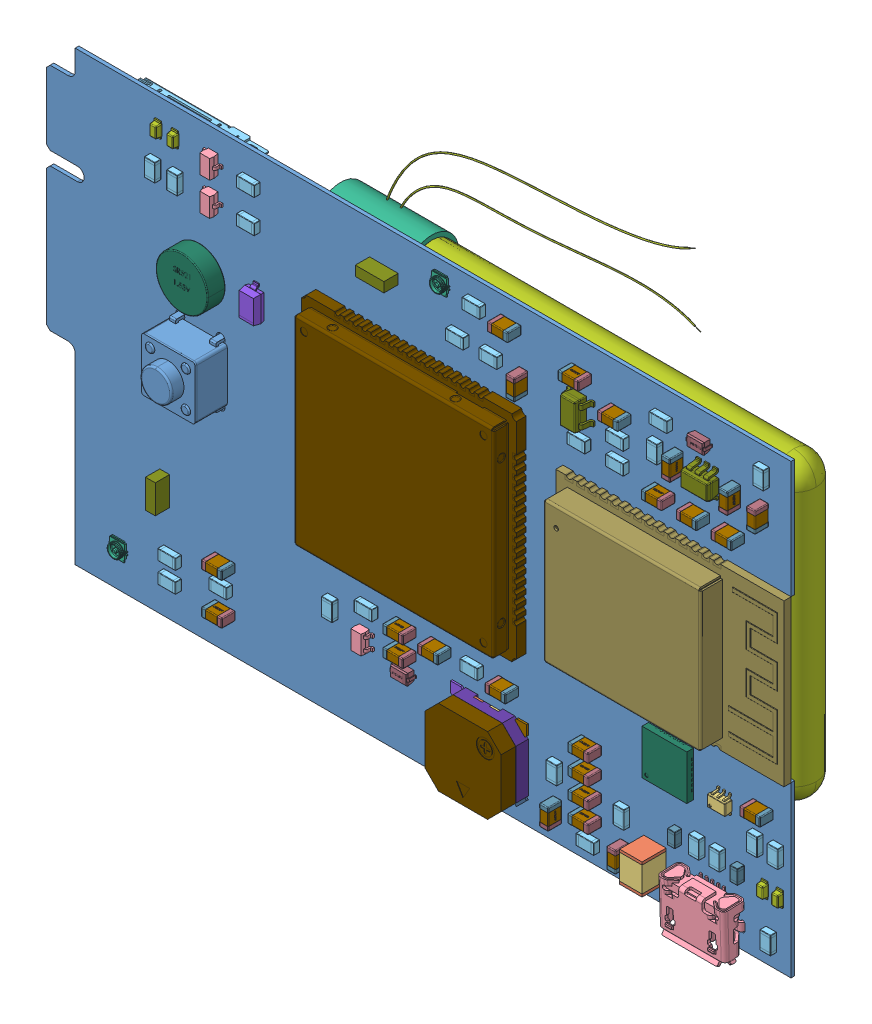
SolidWorks assembly Venato_PCB_v1, configuration Default. Lengths in mm.
Overall size (83.21 61.18 11.57).
389 component instances, 43 part files, 0 mates.
Components (placement in the parent):
- Venato_PCB_v1.step-1: Venato_PCB_v1.step [Default] at origin size (83.21 61.18 11.57)
  - Board.step-1: Board.step [Default] at origin size (83.2 50 0.41)
    - Open CASCADE STEP translator 7.5 1.1.1.step-1: Open CASCADE STEP translator 7.5 1.1.1.step [Default] at (0 0 -0.4115) size (83.2 50 0.41)
  - U6.step-1: U6.step [Default] at origin size (2.8 2.9 1.45)
    - DW01A--3DModel-STEP-56544.step-1: DW01A--3DModel-STEP-56544.step [Default] at (36.6 15.9 -0.4115) x (-1 0 0) z (0 -1 0) size (2.8 1.45 2.9)
  - U10.step-1: U10.step [Default] at origin size (2 2.1 0.99)
    - User Library-SW3dPS-SOT363.step-1: User Library-SW3dPS-SOT363.step [Default] at (26.5 42.9 -1.2115) x (0 1 0) z (-1 0 0) size (2.1 0.99 2)
  - T3.step-1: T3.step [Default] at origin size (2.1 2.1 1)
    - 2N7002H6327XTSA2.step-1: 2N7002H6327XTSA2.step [Default] at (19.7 50.9 0.6) x (0 -1 0) z (-1 0 0) size (2.1 1 2.1)
  - T2.step-1: T2.step [Default] at origin size (2.1 2.1 1)
    - 2N7002H6327XTSA2.step-1: 2N7002H6327XTSA2.step [Default] at (19.7 47.2 0.6) x (0 -1 0) z (-1 0 0) size (2.1 1 2.1)
  - R32.step-1: R32.step [Default] at origin size (2 1.2 0.7)
    - User Library-Chip Resistor2.step-1: User Library-Chip Resistor2.step [Default] at (23.9 50.8999 0) x (1 0 0) z (0 -1 0) size (2 0.7 1.2)
  - R31.step-1: R31.step [Default] at origin size (2 1.2 0.7)
    - User Library-Chip Resistor2.step-1: User Library-Chip Resistor2.step [Default] at (23.9 47.1999 0) x (1 0 0) z (0 -1 0) size (2 0.7 1.2)
  - R30.step-1: R30.step [Default] at origin size (1.2 2 0.7)
    - User Library-Chip Resistor2.step-1: User Library-Chip Resistor2.step [Default] at (15.6999 47.15 0) x (0 -1 0) z (-1 0 0) size (2 0.7 1.2)
  - R29.step-1: R29.step [Default] at origin size (1.2 2 0.7)
    - User Library-Chip Resistor2.step-1: User Library-Chip Resistor2.step [Default] at (13.1999 47.15 0) x (0 -1 0) z (-1 0 0) size (2 0.7 1.2)
  - R28.step-1: R28.step [Default] at origin size (2 1.2 0.7)
    - User Library-Chip Resistor2.step-1: User Library-Chip Resistor2.step [Default] at (15.1 8.0999 0) x (1 0 0) z (0 -1 0) size (2 0.7 1.2)
  - R27.step-1: R27.step [Default] at origin size (2 1.2 0.7)
    - User Library-Chip Resistor2.step-1: User Library-Chip Resistor2.step [Default] at (20.8 10.3999 0) x (1 0 0) z (0 -1 0) size (2 0.7 1.2)
  - R26.step-1: R26.step [Default] at origin size (2 1.2 0.7)
    - User Library-Chip Resistor2.step-1: User Library-Chip Resistor2.step [Default] at (49.1 51.6999 0) x (1 0 0) z (0 -1 0) size (2 0.7 1.2)
  - R25.step-1: R25.step [Default] at origin size (2 1.2 0.7)
    - User Library-Chip Resistor2.step-1: User Library-Chip Resistor2.step [Default] at (51 47.7999 0) x (1 0 0) z (0 -1 0) size (2 0.7 1.2)
  - R24.step-1: R24.step [Default] at origin size (2 1.2 0.7)
    - User Library-Chip Resistor2.step-1: User Library-Chip Resistor2.step [Default] at (15.1 10.3999 0) x (1 0 0) z (0 -1 0) size (2 0.7 1.2)
  - R23.step-1: R23.step [Default] at origin size (2 1.2 0.7)
    - User Library-Chip Resistor2.step-1: User Library-Chip Resistor2.step [Default] at (47.25 47.7999 0) x (1 0 0) z (0 -1 0) size (2 0.7 1.2)
  - J4.step-1: J4.step [Default] at origin size (2 2 0.6)
    - 20579-001E--3DModel-STEP-231308.step-1: 20579-001E--3DModel-STEP-231308.step [Default] at (9.0822 8.1155 0) x (-1 0 0) z (0 1 0) size (2 0.6 2)
  - J3.step-1: J3.step [Default] at origin size (2 2 0.6)
    - 20579-001E--3DModel-STEP-231308.step-1: 20579-001E--3DModel-STEP-231308.step [Default] at (45.0822 51.8155 0) x (-1 0 0) z (0 1 0) size (2 0.6 2)
  - D9.step-1: D9.step [Default] at origin size (0.8 1.7 0.66)
    - User Library-LED SMD 0603 super red.step-1: User Library-LED SMD 0603 super red.step [Default] at (15.4 51 0) x (-1 0 0) z (0 0 1) size (0.8 1.7 0.66)
  - D8.step-1: D8.step [Default] at origin size (0.8 1.7 0.66)
    - User Library-LED SMD 0603 super red.step-1: User Library-LED SMD 0603 super red.step [Default] at (13.5 51 0) x (-1 0 0) z (0 0 1) size (0.8 1.7 0.66)
  - D7.step-1: D7.step [Default] at origin size (1.8 3.9 1.18)
    - User Library-SOD123-1.step-1: User Library-SOD123-1.step [Default] at (24.5 39.675 0) x (0 1 0) z (0 0 1) size (3.9 1.8 1.18)
  - C27.step-1: C27.step [Default] at origin size (2.3 1 1.55)
    - c0805x472j2gacauto.step-1: c0805x472j2gacauto.step [Default] at (-75.9086 23.8522 -42.7482) x (-1 0 0) z (0 0 1) size (2.3 1 1.55)
      - Open CASCADE STEP translator 7.5 1.21.1.1.step-1: Open CASCADE STEP translator 7.5 1.21.1.1.step [Default] at origin size (2.1 0.98 1.53)
      - Open CASCADE STEP translator 7.5 1.21.1.2.step-1: Open CASCADE STEP translator 7.5 1.21.1.2.step [Default] at origin size (0.36 0 0.19)
      - Open CASCADE STEP translator 7.5 1.21.1.3.step-1: Open CASCADE STEP translator 7.5 1.21.1.3.step [Default] at origin size (0.44 0 0.19)
      - Open CASCADE STEP translator 7.5 1.21.1.4.step-1: Open CASCADE STEP translator 7.5 1.21.1.4.step [Default] at origin size (0.23 0 0.19)
      - Open CASCADE STEP translator 7.5 1.21.1.5.step-1: Open CASCADE STEP translator 7.5 1.21.1.5.step [Default] at origin size (0.5 1 1.55)
      - Open CASCADE STEP translator 7.5 1.21.1.6.step-1: Open CASCADE STEP translator 7.5 1.21.1.6.step [Default] at origin size (0.5 1 1.55)
  - C26.step-1: C26.step [Default] at origin size (2.3 1 1.55)
    - c0805x472j2gacauto.step-1: c0805x472j2gacauto.step [Default] at (117.8086 -3.0522 -42.7482) size (2.3 1 1.55)
      - Open CASCADE STEP translator 7.5 1.21.1.1.step-1: Open CASCADE STEP translator 7.5 1.21.1.1.step [Default] at origin size (2.1 0.98 1.53)
      - Open CASCADE STEP translator 7.5 1.21.1.2.step-1: Open CASCADE STEP translator 7.5 1.21.1.2.step [Default] at origin size (0.36 0 0.19)
      - Open CASCADE STEP translator 7.5 1.21.1.3.step-1: Open CASCADE STEP translator 7.5 1.21.1.3.step [Default] at origin size (0.44 0 0.19)
      - Open CASCADE STEP translator 7.5 1.21.1.4.step-1: Open CASCADE STEP translator 7.5 1.21.1.4.step [Default] at origin size (0.23 0 0.19)
      - Open CASCADE STEP translator 7.5 1.21.1.5.step-1: Open CASCADE STEP translator 7.5 1.21.1.5.step [Default] at origin size (0.5 1 1.55)
      - Open CASCADE STEP translator 7.5 1.21.1.6.step-1: Open CASCADE STEP translator 7.5 1.21.1.6.step [Default] at origin size (0.5 1 1.55)
  - C25.step-1: C25.step [Default] at origin size (2.3 1 1.55)
    - c0805x472j2gacauto.step-1: c0805x472j2gacauto.step [Default] at (-43.9586 62.8522 -42.7482) x (-1 0 0) z (0 0 1) size (2.3 1 1.55)
      - Open CASCADE STEP translator 7.5 1.21.1.1.step-1: Open CASCADE STEP translator 7.5 1.21.1.1.step [Default] at origin size (2.1 0.98 1.53)
      - Open CASCADE STEP translator 7.5 1.21.1.2.step-1: Open CASCADE STEP translator 7.5 1.21.1.2.step [Default] at origin size (0.36 0 0.19)
      - Open CASCADE STEP translator 7.5 1.21.1.3.step-1: Open CASCADE STEP translator 7.5 1.21.1.3.step [Default] at origin size (0.44 0 0.19)
      - Open CASCADE STEP translator 7.5 1.21.1.4.step-1: Open CASCADE STEP translator 7.5 1.21.1.4.step [Default] at origin size (0.23 0 0.19)
      - Open CASCADE STEP translator 7.5 1.21.1.5.step-1: Open CASCADE STEP translator 7.5 1.21.1.5.step [Default] at origin size (0.5 1 1.55)
      - Open CASCADE STEP translator 7.5 1.21.1.6.step-1: Open CASCADE STEP translator 7.5 1.21.1.6.step [Default] at origin size (0.5 1 1.55)
  - C24.step-1: C24.step [Default] at origin size (1 2.3 1.55)
    - c0805x472j2gacauto.step-1: c0805x472j2gacauto.step [Default] at (65.4522 143.8586 -42.7482) x (0 1 0) z (0 0 1) size (2.3 1 1.55)
      - Open CASCADE STEP translator 7.5 1.21.1.1.step-1: Open CASCADE STEP translator 7.5 1.21.1.1.step [Default] at origin size (2.1 0.98 1.53)
      - Open CASCADE STEP translator 7.5 1.21.1.2.step-1: Open CASCADE STEP translator 7.5 1.21.1.2.step [Default] at origin size (0.36 0 0.19)
      - Open CASCADE STEP translator 7.5 1.21.1.3.step-1: Open CASCADE STEP translator 7.5 1.21.1.3.step [Default] at origin size (0.44 0 0.19)
      - Open CASCADE STEP translator 7.5 1.21.1.4.step-1: Open CASCADE STEP translator 7.5 1.21.1.4.step [Default] at origin size (0.23 0 0.19)
      - Open CASCADE STEP translator 7.5 1.21.1.5.step-1: Open CASCADE STEP translator 7.5 1.21.1.5.step [Default] at origin size (0.5 1 1.55)
      - Open CASCADE STEP translator 7.5 1.21.1.6.step-1: Open CASCADE STEP translator 7.5 1.21.1.6.step [Default] at origin size (0.5 1 1.55)
  - BAT1.step-1: BAT1.step [Default] at origin size (5.8 5.8 2.15)
    - User Library-SR521.step-1: User Library-SR521.step [Default] at (18.3 39.5 2.2) x (-1 0 0) z (0 0 -1) size (5.8 5.8 2.15)
  - ANT2.step-1: ANT2.step [Default] at origin size (1.1 3.2 1.6)
    - w3043.step-1: w3043.step [Default] at (13.65 16.5 0.8) x (0 -1 0) z (0 0 1) size (3.2 1.1 1.6)
  - ANT1.step-1: ANT1.step [Default] at origin size (3.2 1.1 1.6)
    - w3043.step-1: w3043.step [Default] at (38.7 49.25 0.8) x (1 0 0) z (0 0 1) size (3.2 1.1 1.6)
  - B1.step-1: B1.step [Default] at origin size (8.5 8.5 3.05)
    - CMT-8503-87_90.step-1: CMT-8503-87_90.step [Default] at (50.6 9.8 0) x (1 0 0) z (0 0 1) size (8.5 8.5 3.05)
      - CaseBody.step-1: CaseBody.step [Default] at (0 0 0.01) size (8.5 8.5 2.5)
      - CoverBody.step-1: CoverBody.step [Default] at (0 0 1.42) size (8.5 8.5 1.64)
      - MembraneBody.step-1: MembraneBody.step [Default] at (0 0 1.91) size (7.9 7.9 0.3)
      - Plate1Body.step-1: Plate1Body.step [Default] at (0 0 0.51) size (1 0.75 0.2)
      - Plate2Body.step-1: Plate2Body.step [Default] at (0 0 0.51) size (1 0.75 0.2)
      - Plate3Body.step-1: Plate3Body.step [Default] at (0 0 0.51) size (1 0.75 0.2)
      - Plate4Body.step-1: Plate4Body.step [Default] at (0 0 0.51) size (1 0.75 0.2)
      - Plate5Body.step-1: Plate5Body.step [Default] at (0 0 0.51) size (0.5 0.5 0.2)
      - Plate6Body.step-1: Plate6Body.step [Default] at (0 0 0.51) size (0.5 0.5 0.2)
      - Pin1Body.step-1: Pin1Body.step [Default] at (0 0 0.21) size (1.63 1.63 0.2)
      - Pin2Body.step-1: Pin2Body.step [Default] at (0 0 0.21) size (1.63 1.63 0.2)
      - Pin3Body.step-1: Pin3Body.step [Default] at (0 0 0.21) size (1.63 1.63 0.2)
      - Pin4Body.step-1: Pin4Body.step [Default] at (0 0 0.21) size (1.63 1.63 0.2)
  - U1.step-1: U1.step [Default] at origin size (25.5 18 3.25)
    - ESP32-WROOM-32E (16MB)--3DModel-STEP-269445.step-1: ESP32-WROOM-32E (16MB)--3DModel-STEP-269445.step [Default] at (71.46 32 0) x (0 -1 0) z (-1 0 0) size (18 3.25 25.5)
  - D3.step-1: D3.step [Default] at origin size (2.51 1.26 1)
    - User Library-SOD323.step-1: User Library-SOD323.step [Default] at (41.2 12.925 0) x (-1 0 0) z (0 0 1) size (2.51 1.26 1)
  - Z2.step-1: Z2.step [Default] at origin size (0.84 1.6 0.8)
    - R0603.step-1: R0603.step [Default] at (71.18 11.6874 0.4127) x (0 1 0) z (0 0 -1) size (1.6 0.84 0.8)
  - Z1.step-1: Z1.step [Default] at origin size (0.84 1.6 0.8)
    - R0603.step-1: R0603.step [Default] at (78.18 11.6374 0.4127) x (0 1 0) z (0 0 -1) size (1.6 0.84 0.8)
  - U9.step-1: U9.step [Default] at origin size (2 2.1 0.99)
    - User Library-SW3dPS-SOT363.step-1: User Library-SW3dPS-SOT363.step [Default] at (76.8 17.6 0.8) x (0 1 0) z (1 0 0) size (2.1 0.99 2)
  - U8.step-1: U8.step [Default] at origin size (5.02 5.02 0.75)
    - cp2102n-a01-gqfn28.step-1: cp2102n-a01-gqfn28.step [Default] at (68.3 18.4 0) x (1 0 0) z (0 -1 0) size (5.02 0.75 5.02)
  - U7.step-1: U7.step [Default] at origin size (2.8 2.9 1.45)
    - DW01A--3DModel-STEP-56544.step-1: DW01A--3DModel-STEP-56544.step [Default] at (41.3 13.1 -0.4115) x (-1 0 0) z (0 -1 0) size (2.8 1.45 2.9)
  - U5.step-1: U5.step [Default] at origin size (3.03 3.05 1.62)
    - User Library-TPS79333DBVR.step-1: User Library-TPS79333DBVR.step [Default] at (60.7864 47.75 1.2) x (0 -1 0) z (-1 0 0) size (3.05 1.62 3.03)
  - U4.step-1: U4.step [Default] at origin size (3.05 3.03 1.62)
    - User Library-TPS79333DBVR.step-1: User Library-TPS79333DBVR.step [Default] at (74.9 47.8636 1.2) x (-1 0 0) z (0 1 0) size (3.05 1.62 3.03)
  - U3.step-1: U3.step [Default] at origin size (6.22 5.01 1.87)
    - SOP-8.step-1: SOP-8.step [Default] at (39 8.2 -0.4115) x (0 -1 0) z (1 0 0) size (5.01 1.87 6.22)
  - U2.step-1: U2.step [Default] at origin size (24 24 2.8)
    - SIM808--3DModel-STEP-56544.step-1: SIM808--3DModel-STEP-56544.step [Default] at (42.6 32.2 0) x (0 1 0) z (1 0 0) size (24 2.8 24)
  - T1.step-1: T1.step [Default] at origin size (2.1 2.1 1)
    - 2N7002H6327XTSA2.step-1: 2N7002H6327XTSA2.step [Default] at (36.6 13.3 0.6) x (0 1 0) z (1 0 0) size (2.1 1 2.1)
  - SW2.step-1: SW2.step [Default] at origin size (5.99 7.8 8.51)
    - User Library-FSM4JLH(1825910-5).step-1: User Library-FSM4JLH(1825910-5).step [Default] at (18.2 30.9 0) x (0 1 0) z (0 0 1) size (7.8 5.99 8.51)
  - R22.step-1: R22.step [Default] at origin size (1.2 2 0.7)
    - User Library-Chip Resistor2.step-1: User Library-Chip Resistor2.step [Default] at (65.5999 10.7 0) x (0 -1 0) z (-1 0 0) size (2 0.7 1.2)
  - R21.step-1: R21.step [Default] at origin size (1.2 2 0.7)
    - User Library-Chip Resistor2.step-1: User Library-Chip Resistor2.step [Default] at (82.0001 6.75 0) x (0 1 0) z (1 0 0) size (2 0.7 1.2)
  - R20.step-1: R20.step [Default] at origin size (1.2 2 0.7)
    - User Library-Chip Resistor2.step-1: User Library-Chip Resistor2.step [Default] at (76.2999 12 0) x (0 -1 0) z (-1 0 0) size (2 0.7 1.2)
  - R19.step-1: R19.step [Default] at origin size (1.2 2 0.7)
    - User Library-Chip Resistor2.step-1: User Library-Chip Resistor2.step [Default] at (73.9999 12 0) x (0 -1 0) z (-1 0 0) size (2 0.7 1.2)
  - R18.step-1: R18.step [Default] at origin size (2 1.2 0.7)
    - User Library-Chip Resistor2.step-1: User Library-Chip Resistor2.step [Default] at (61.85 6.1999 0) x (1 0 0) z (0 -1 0) size (2 0.7 1.2)
  - R17.step-1: R17.step [Default] at origin size (1.2 2 0.7)
    - User Library-Chip Resistor2.step-1: User Library-Chip Resistor2.step [Default] at (82.7999 15.5 0) x (0 -1 0) z (-1 0 0) size (2 0.7 1.2)
  - R16.step-1: R16.step [Default] at origin size (1.2 2 0.7)
    - User Library-Chip Resistor2.step-1: User Library-Chip Resistor2.step [Default] at (80.4999 15.5 0) x (0 -1 0) z (-1 0 0) size (2 0.7 1.2)
  - R15.step-1: R15.step [Default] at origin size (2 1.2 0.7)
    - User Library-Chip Resistor2.step-1: User Library-Chip Resistor2.step [Default] at (41.3 16.6001 -0.4115) x (1 0 0) z (0 1 0) size (2 0.7 1.2)
  - R14.step-1: R14.step [Default] at origin size (2 1.2 0.7)
    - User Library-Chip Resistor2.step-1: User Library-Chip Resistor2.step [Default] at (36.7 12.6999 -0.4115) x (-1 0 0) z (0 -1 0) size (2 0.7 1.2)
  - R13.step-1: R13.step [Default] at origin size (2 1.2 0.7)
    - User Library-Chip Resistor2.step-1: User Library-Chip Resistor2.step [Default] at (65.15 44.5499 0) x (1 0 0) z (0 -1 0) size (2 0.7 1.2)
  - R12.step-1: R12.step [Default] at origin size (1.2 2 0.7)
    - User Library-Chip Resistor2.step-1: User Library-Chip Resistor2.step [Default] at (69.3001 47.9 0) x (0 1 0) z (1 0 0) size (2 0.7 1.2)
  - R11.step-1: R11.step [Default] at origin size (2 1.2 0.7)
    - User Library-Chip Resistor2.step-1: User Library-Chip Resistor2.step [Default] at (60.85 44.5499 0) x (1 0 0) z (0 -1 0) size (2 0.7 1.2)
  - R10.step-1: R10.step [Default] at origin size (2 1.2 0.7)
    - User Library-Chip Resistor2.step-1: User Library-Chip Resistor2.step [Default] at (65.15 46.9499 0) x (1 0 0) z (0 -1 0) size (2 0.7 1.2)
  - R9.step-1: R9.step [Default] at origin size (2 1.2 0.7)
    - User Library-Chip Resistor2.step-1: User Library-Chip Resistor2.step [Default] at (70 51.1001 0) x (-1 0 0) z (0 1 0) size (2 0.7 1.2)
  - R8.step-1: R8.step [Default] at origin size (1.2 2 0.7)
    - User Library-Chip Resistor2.step-1: User Library-Chip Resistor2.step [Default] at (45.0001 7.65 -0.4115) x (0 -1 0) z (1 0 0) size (2 0.7 1.2)
  - R7.step-1: R7.step [Default] at origin size (1.2 2 0.7)
    - User Library-Chip Resistor2.step-1: User Library-Chip Resistor2.step [Default] at (30.5841 7.4 -0.4115) x (0 -1 0) z (1 0 0) size (2 0.7 1.2)
  - R6.step-1: R6.step [Default] at origin size (1.2 2 0.7)
    - User Library-Chip Resistor2.step-1: User Library-Chip Resistor2.step [Default] at (32.8841 7.4 -0.4115) x (0 -1 0) z (1 0 0) size (2 0.7 1.2)
  - R5.step-1: R5.step [Default] at origin size (2 1.2 0.7)
    - User Library-Chip Resistor2.step-1: User Library-Chip Resistor2.step [Default] at (48.85 16.6001 0) x (-1 0 0) z (0 1 0) size (2 0.7 1.2)
  - R4.step-1: R4.step [Default] at origin size (2 1.2 0.7)
    - User Library-Chip Resistor2.step-1: User Library-Chip Resistor2.step [Default] at (37.05 16.4001 0) x (-1 0 0) z (0 1 0) size (2 0.7 1.2)
  - R3.step-1: R3.step [Default] at origin size (1.2 2 0.7)
    - User Library-Chip Resistor2.step-1: User Library-Chip Resistor2.step [Default] at (33.0001 14.5 0) x (0 1 0) z (1 0 0) size (2 0.7 1.2)
  - R2.step-1: R2.step [Default] at origin size (1.2 2 0.7)
    - User Library-Chip Resistor2.step-1: User Library-Chip Resistor2.step [Default] at (81.2001 51.35 0) x (0 1 0) z (1 0 0) size (2 0.7 1.2)
  - R1.step-1: R1.step [Default] at origin size (1.2 2 0.7)
    - User Library-Chip Resistor2.step-1: User Library-Chip Resistor2.step [Default] at (58.0999 11.25 0) x (0 -1 0) z (-1 0 0) size (2 0.7 1.2)
  - L1.step-1: L1.step [Default] at origin size (2.5 3.4 2.71)
    - 6240506192.step-1: 6240506192.step [Default] at (69 9.55 -0.005) size (2.5 0.3 2.71)
      - Extruded.step-1: Extruded.step [Default] at origin size (2.5 0.3 2.71)
    - 6240506192.step-2: 6240506192.step [Default] at (69 6.45 -0.005) size (2.5 0.3 2.71)
      - Extruded.step-1: Extruded.step [Default] at origin size (2.5 0.3 2.71)
    - 6240505952.step-1: 6240505952.step [Default] at (69 8 -0.005) size (2.5 2.8 2.71)
      - Extruded-0.step-1: Extruded-0.step [Default] at origin size (2.5 2.8 2.71)
  - J2.step-1: J2.step [Default] at origin size (7.87 5.84 3.81)
    - 10118193-0001lfc.step-1: 10118193-0001lfc.step [Default] at (-22.5035 9.5518 -0.2912) x (1 0 0) z (0 -0.99938 -0.035196) size (7.87 3.61 5.71)
  - J1.step-1: J1.step [Default] at origin size (16.96 13.85 1.5)
    - 78800-0001.step-1: 78800-0001.step [Default] at (15.7 46.7 -0.4115) x (-1 0 0) z (0 0 -1) size (16.96 13.85 1.5)
  - FB2.step-1: FB2.step [Default] at origin size (2.3 1 1.55)
    - c0805x472j2gacauto.step-1: c0805x472j2gacauto.step [Default] at (158.7586 -0.2522 -42.7482) size (2.3 1 1.55)
      - Open CASCADE STEP translator 7.5 1.21.1.1.step-1: Open CASCADE STEP translator 7.5 1.21.1.1.step [Default] at origin size (2.1 0.98 1.53)
      - Open CASCADE STEP translator 7.5 1.21.1.2.step-1: Open CASCADE STEP translator 7.5 1.21.1.2.step [Default] at origin size (0.36 0 0.19)
      - Open CASCADE STEP translator 7.5 1.21.1.3.step-1: Open CASCADE STEP translator 7.5 1.21.1.3.step [Default] at origin size (0.44 0 0.19)
      - Open CASCADE STEP translator 7.5 1.21.1.4.step-1: Open CASCADE STEP translator 7.5 1.21.1.4.step [Default] at origin size (0.23 0 0.19)
      - Open CASCADE STEP translator 7.5 1.21.1.5.step-1: Open CASCADE STEP translator 7.5 1.21.1.5.step [Default] at origin size (0.5 1 1.55)
      - Open CASCADE STEP translator 7.5 1.21.1.6.step-1: Open CASCADE STEP translator 7.5 1.21.1.6.step [Default] at origin size (0.5 1 1.55)
  - FB1.step-1: FB1.step [Default] at origin size (2.3 1 1.55)
    - c0805x472j2gacauto.step-1: c0805x472j2gacauto.step [Default] at (-18.9586 55.2022 -42.7482) x (-1 0 0) z (0 0 1) size (2.3 1 1.55)
      - Open CASCADE STEP translator 7.5 1.21.1.1.step-1: Open CASCADE STEP translator 7.5 1.21.1.1.step [Default] at origin size (2.1 0.98 1.53)
      - Open CASCADE STEP translator 7.5 1.21.1.2.step-1: Open CASCADE STEP translator 7.5 1.21.1.2.step [Default] at origin size (0.36 0 0.19)
      - Open CASCADE STEP translator 7.5 1.21.1.3.step-1: Open CASCADE STEP translator 7.5 1.21.1.3.step [Default] at origin size (0.44 0 0.19)
      - Open CASCADE STEP translator 7.5 1.21.1.4.step-1: Open CASCADE STEP translator 7.5 1.21.1.4.step [Default] at origin size (0.23 0 0.19)
      - Open CASCADE STEP translator 7.5 1.21.1.5.step-1: Open CASCADE STEP translator 7.5 1.21.1.5.step [Default] at origin size (0.5 1 1.55)
      - Open CASCADE STEP translator 7.5 1.21.1.6.step-1: Open CASCADE STEP translator 7.5 1.21.1.6.step [Default] at origin size (0.5 1 1.55)
  - D6.step-1: D6.step [Default] at origin size (0.8 1.7 0.66)
    - User Library-LED SMD 0603 super red.step-1: User Library-LED SMD 0603 super red.step [Default] at (83 11.3 0) x (-1 0 0) z (0 0 1) size (0.8 1.7 0.66)
  - D5.step-1: D5.step [Default] at origin size (0.8 1.7 0.66)
    - User Library-LED SMD 0603 super red.step-1: User Library-LED SMD 0603 super red.step [Default] at (81.3 11.3 0) x (-1 0 0) z (0 0 1) size (0.8 1.7 0.66)
  - D4.step-1: D4.step [Default] at origin size (2.51 1.26 1)
    - User Library-SOD323.step-1: User Library-SOD323.step [Default] at (74.3192 50.575 0) size (2.51 1.26 1)
  - D2.step-1: D2.step [Default] at origin size (0.8 1.7 0.66)
    - User Library-LED SMD 0603 super red.step-1: User Library-LED SMD 0603 super red.step [Default] at (32.584 11.15 -0.4115) x (1 0 0) z (0 0 -1) size (0.8 1.7 0.66)
  - D1.step-1: D1.step [Default] at origin size (0.8 1.7 0.66)
    - User Library-LED SMD 0603 super red.step-1: User Library-LED SMD 0603 super red.step [Default] at (30.884 11.15 -0.4115) x (1 0 0) z (0 0 -1) size (0.8 1.7 0.66)
  - C23.step-1: C23.step [Default] at origin size (1 2.3 1.55)
    - c0805x472j2gacauto.step-1: c0805x472j2gacauto.step [Default] at (46.9478 -89.5086 -42.7482) x (0 -1 0) z (0 0 1) size (2.3 1 1.55)
      - Open CASCADE STEP translator 7.5 1.21.1.1.step-1: Open CASCADE STEP translator 7.5 1.21.1.1.step [Default] at origin size (2.1 0.98 1.53)
      - Open CASCADE STEP translator 7.5 1.21.1.2.step-1: Open CASCADE STEP translator 7.5 1.21.1.2.step [Default] at origin size (0.36 0 0.19)
      - Open CASCADE STEP translator 7.5 1.21.1.3.step-1: Open CASCADE STEP translator 7.5 1.21.1.3.step [Default] at origin size (0.44 0 0.19)
      - Open CASCADE STEP translator 7.5 1.21.1.4.step-1: Open CASCADE STEP translator 7.5 1.21.1.4.step [Default] at origin size (0.23 0 0.19)
      - Open CASCADE STEP translator 7.5 1.21.1.5.step-1: Open CASCADE STEP translator 7.5 1.21.1.5.step [Default] at origin size (0.5 1 1.55)
      - Open CASCADE STEP translator 7.5 1.21.1.6.step-1: Open CASCADE STEP translator 7.5 1.21.1.6.step [Default] at origin size (0.5 1 1.55)
  - C22.step-1: C22.step [Default] at origin size (1 2.3 1.55)
    - c0805x472j2gacauto.step-1: c0805x472j2gacauto.step [Default] at (76.7522 103.8086 -42.7482) x (0 1 0) z (0 0 1) size (2.3 1 1.55)
      - Open CASCADE STEP translator 7.5 1.21.1.1.step-1: Open CASCADE STEP translator 7.5 1.21.1.1.step [Default] at origin size (2.1 0.98 1.53)
      - Open CASCADE STEP translator 7.5 1.21.1.2.step-1: Open CASCADE STEP translator 7.5 1.21.1.2.step [Default] at origin size (0.36 0 0.19)
      - Open CASCADE STEP translator 7.5 1.21.1.3.step-1: Open CASCADE STEP translator 7.5 1.21.1.3.step [Default] at origin size (0.44 0 0.19)
      - Open CASCADE STEP translator 7.5 1.21.1.4.step-1: Open CASCADE STEP translator 7.5 1.21.1.4.step [Default] at origin size (0.23 0 0.19)
      - Open CASCADE STEP translator 7.5 1.21.1.5.step-1: Open CASCADE STEP translator 7.5 1.21.1.5.step [Default] at origin size (0.5 1 1.55)
      - Open CASCADE STEP translator 7.5 1.21.1.6.step-1: Open CASCADE STEP translator 7.5 1.21.1.6.step [Default] at origin size (0.5 1 1.55)
  - C21.step-1: C21.step [Default] at origin size (2.3 1 1.55)
    - c0805x472j2gacauto.step-1: c0805x472j2gacauto.step [Default] at (158.7586 4.3478 -42.7482) size (2.3 1 1.55)
      - Open CASCADE STEP translator 7.5 1.21.1.1.step-1: Open CASCADE STEP translator 7.5 1.21.1.1.step [Default] at origin size (2.1 0.98 1.53)
      - Open CASCADE STEP translator 7.5 1.21.1.2.step-1: Open CASCADE STEP translator 7.5 1.21.1.2.step [Default] at origin size (0.36 0 0.19)
      - Open CASCADE STEP translator 7.5 1.21.1.3.step-1: Open CASCADE STEP translator 7.5 1.21.1.3.step [Default] at origin size (0.44 0 0.19)
      - Open CASCADE STEP translator 7.5 1.21.1.4.step-1: Open CASCADE STEP translator 7.5 1.21.1.4.step [Default] at origin size (0.23 0 0.19)
      - Open CASCADE STEP translator 7.5 1.21.1.5.step-1: Open CASCADE STEP translator 7.5 1.21.1.5.step [Default] at origin size (0.5 1 1.55)
      - Open CASCADE STEP translator 7.5 1.21.1.6.step-1: Open CASCADE STEP translator 7.5 1.21.1.6.step [Default] at origin size (0.5 1 1.55)
  - C20.step-1: C20.step [Default] at origin size (2.3 1 1.55)
    - c0805x472j2gacauto.step-1: c0805x472j2gacauto.step [Default] at (158.7586 2.0478 -42.7482) size (2.3 1 1.55)
      - Open CASCADE STEP translator 7.5 1.21.1.1.step-1: Open CASCADE STEP translator 7.5 1.21.1.1.step [Default] at origin size (2.1 0.98 1.53)
      - Open CASCADE STEP translator 7.5 1.21.1.2.step-1: Open CASCADE STEP translator 7.5 1.21.1.2.step [Default] at origin size (0.36 0 0.19)
      - Open CASCADE STEP translator 7.5 1.21.1.3.step-1: Open CASCADE STEP translator 7.5 1.21.1.3.step [Default] at origin size (0.44 0 0.19)
      - Open CASCADE STEP translator 7.5 1.21.1.4.step-1: Open CASCADE STEP translator 7.5 1.21.1.4.step [Default] at origin size (0.23 0 0.19)
      - Open CASCADE STEP translator 7.5 1.21.1.5.step-1: Open CASCADE STEP translator 7.5 1.21.1.5.step [Default] at origin size (0.5 1 1.55)
      - Open CASCADE STEP translator 7.5 1.21.1.6.step-1: Open CASCADE STEP translator 7.5 1.21.1.6.step [Default] at origin size (0.5 1 1.55)
  - C19.step-1: C19.step [Default] at origin size (2.3 1 1.55)
    - c0805x472j2gacauto.step-1: c0805x472j2gacauto.step [Default] at (158.7586 -2.5522 -42.7482) size (2.3 1 1.55)
      - Open CASCADE STEP translator 7.5 1.21.1.1.step-1: Open CASCADE STEP translator 7.5 1.21.1.1.step [Default] at origin size (2.1 0.98 1.53)
      - Open CASCADE STEP translator 7.5 1.21.1.2.step-1: Open CASCADE STEP translator 7.5 1.21.1.2.step [Default] at origin size (0.36 0 0.19)
      - Open CASCADE STEP translator 7.5 1.21.1.3.step-1: Open CASCADE STEP translator 7.5 1.21.1.3.step [Default] at origin size (0.44 0 0.19)
      - Open CASCADE STEP translator 7.5 1.21.1.4.step-1: Open CASCADE STEP translator 7.5 1.21.1.4.step [Default] at origin size (0.23 0 0.19)
      - Open CASCADE STEP translator 7.5 1.21.1.5.step-1: Open CASCADE STEP translator 7.5 1.21.1.5.step [Default] at origin size (0.5 1 1.55)
      - Open CASCADE STEP translator 7.5 1.21.1.6.step-1: Open CASCADE STEP translator 7.5 1.21.1.6.step [Default] at origin size (0.5 1 1.55)
  - C18.step-1: C18.step [Default] at origin size (1 2.3 1.55)
    - c0805x472j2gacauto.step-1: c0805x472j2gacauto.step [Default] at (-5.5522 143.3586 42.3367) x (0 1 0) z (0 0 -1) size (2.3 1 1.55)
      - Open CASCADE STEP translator 7.5 1.21.1.1.step-1: Open CASCADE STEP translator 7.5 1.21.1.1.step [Default] at origin size (2.1 0.98 1.53)
      - Open CASCADE STEP translator 7.5 1.21.1.2.step-1: Open CASCADE STEP translator 7.5 1.21.1.2.step [Default] at origin size (0.36 0 0.19)
      - Open CASCADE STEP translator 7.5 1.21.1.3.step-1: Open CASCADE STEP translator 7.5 1.21.1.3.step [Default] at origin size (0.44 0 0.19)
      - Open CASCADE STEP translator 7.5 1.21.1.4.step-1: Open CASCADE STEP translator 7.5 1.21.1.4.step [Default] at origin size (0.23 0 0.19)
      - Open CASCADE STEP translator 7.5 1.21.1.5.step-1: Open CASCADE STEP translator 7.5 1.21.1.5.step [Default] at origin size (0.5 1 1.55)
      - Open CASCADE STEP translator 7.5 1.21.1.6.step-1: Open CASCADE STEP translator 7.5 1.21.1.6.step [Default] at origin size (0.5 1 1.55)
  - C17.step-1: C17.step [Default] at origin size (2.3 1 1.55)
    - c0805x472j2gacauto.step-1: c0805x472j2gacauto.step [Default] at (-70.3586 39.8478 42.3367) x (-1 0 0) z (0 0 -1) size (2.3 1 1.55)
      - Open CASCADE STEP translator 7.5 1.21.1.1.step-1: Open CASCADE STEP translator 7.5 1.21.1.1.step [Default] at origin size (2.1 0.98 1.53)
      - Open CASCADE STEP translator 7.5 1.21.1.2.step-1: Open CASCADE STEP translator 7.5 1.21.1.2.step [Default] at origin size (0.36 0 0.19)
      - Open CASCADE STEP translator 7.5 1.21.1.3.step-1: Open CASCADE STEP translator 7.5 1.21.1.3.step [Default] at origin size (0.44 0 0.19)
      - Open CASCADE STEP translator 7.5 1.21.1.4.step-1: Open CASCADE STEP translator 7.5 1.21.1.4.step [Default] at origin size (0.23 0 0.19)
      - Open CASCADE STEP translator 7.5 1.21.1.5.step-1: Open CASCADE STEP translator 7.5 1.21.1.5.step [Default] at origin size (0.5 1 1.55)
      - Open CASCADE STEP translator 7.5 1.21.1.6.step-1: Open CASCADE STEP translator 7.5 1.21.1.6.step [Default] at origin size (0.5 1 1.55)
  - C16.step-1: C16.step [Default] at origin size (2.3 1 1.55)
    - c0805x472j2gacauto.step-1: c0805x472j2gacauto.step [Default] at (-70.3586 37.5478 42.3367) x (-1 0 0) z (0 0 -1) size (2.3 1 1.55)
      - Open CASCADE STEP translator 7.5 1.21.1.1.step-1: Open CASCADE STEP translator 7.5 1.21.1.1.step [Default] at origin size (2.1 0.98 1.53)
      - Open CASCADE STEP translator 7.5 1.21.1.2.step-1: Open CASCADE STEP translator 7.5 1.21.1.2.step [Default] at origin size (0.36 0 0.19)
      - Open CASCADE STEP translator 7.5 1.21.1.3.step-1: Open CASCADE STEP translator 7.5 1.21.1.3.step [Default] at origin size (0.44 0 0.19)
      - Open CASCADE STEP translator 7.5 1.21.1.4.step-1: Open CASCADE STEP translator 7.5 1.21.1.4.step [Default] at origin size (0.23 0 0.19)
      - Open CASCADE STEP translator 7.5 1.21.1.5.step-1: Open CASCADE STEP translator 7.5 1.21.1.5.step [Default] at origin size (0.5 1 1.55)
      - Open CASCADE STEP translator 7.5 1.21.1.6.step-1: Open CASCADE STEP translator 7.5 1.21.1.6.step [Default] at origin size (0.5 1 1.55)
  - C15.step-1: C15.step [Default] at origin size (2.3 1 1.55)
    - c0805x472j2gacauto.step-1: c0805x472j2gacauto.step [Default] at (-70.3586 35.2478 42.3367) x (-1 0 0) z (0 0 -1) size (2.3 1 1.55)
      - Open CASCADE STEP translator 7.5 1.21.1.1.step-1: Open CASCADE STEP translator 7.5 1.21.1.1.step [Default] at origin size (2.1 0.98 1.53)
      - Open CASCADE STEP translator 7.5 1.21.1.2.step-1: Open CASCADE STEP translator 7.5 1.21.1.2.step [Default] at origin size (0.36 0 0.19)
      - Open CASCADE STEP translator 7.5 1.21.1.3.step-1: Open CASCADE STEP translator 7.5 1.21.1.3.step [Default] at origin size (0.44 0 0.19)
      - Open CASCADE STEP translator 7.5 1.21.1.4.step-1: Open CASCADE STEP translator 7.5 1.21.1.4.step [Default] at origin size (0.23 0 0.19)
      - Open CASCADE STEP translator 7.5 1.21.1.5.step-1: Open CASCADE STEP translator 7.5 1.21.1.5.step [Default] at origin size (0.5 1 1.55)
      - Open CASCADE STEP translator 7.5 1.21.1.6.step-1: Open CASCADE STEP translator 7.5 1.21.1.6.step [Default] at origin size (0.5 1 1.55)
  - C14.step-1: C14.step [Default] at origin size (1 2.3 1.55)
    - c0805x472j2gacauto.step-1: c0805x472j2gacauto.step [Default] at (43.4522 -81.5586 42.3367) x (0 -1 0) z (0 0 -1) size (2.3 1 1.55)
      - Open CASCADE STEP translator 7.5 1.21.1.1.step-1: Open CASCADE STEP translator 7.5 1.21.1.1.step [Default] at origin size (2.1 0.98 1.53)
      - Open CASCADE STEP translator 7.5 1.21.1.2.step-1: Open CASCADE STEP translator 7.5 1.21.1.2.step [Default] at origin size (0.36 0 0.19)
      - Open CASCADE STEP translator 7.5 1.21.1.3.step-1: Open CASCADE STEP translator 7.5 1.21.1.3.step [Default] at origin size (0.44 0 0.19)
      - Open CASCADE STEP translator 7.5 1.21.1.4.step-1: Open CASCADE STEP translator 7.5 1.21.1.4.step [Default] at origin size (0.23 0 0.19)
      - Open CASCADE STEP translator 7.5 1.21.1.5.step-1: Open CASCADE STEP translator 7.5 1.21.1.5.step [Default] at origin size (0.5 1 1.55)
      - Open CASCADE STEP translator 7.5 1.21.1.6.step-1: Open CASCADE STEP translator 7.5 1.21.1.6.step [Default] at origin size (0.5 1 1.55)
  - C13.step-1: C13.step [Default] at origin size (2.3 1 1.55)
    - c0805x472j2gacauto.step-1: c0805x472j2gacauto.step [Default] at (157.6586 39.7978 -42.7482) size (2.3 1 1.55)
      - Open CASCADE STEP translator 7.5 1.21.1.1.step-1: Open CASCADE STEP translator 7.5 1.21.1.1.step [Default] at origin size (2.1 0.98 1.53)
      - Open CASCADE STEP translator 7.5 1.21.1.2.step-1: Open CASCADE STEP translator 7.5 1.21.1.2.step [Default] at origin size (0.36 0 0.19)
      - Open CASCADE STEP translator 7.5 1.21.1.3.step-1: Open CASCADE STEP translator 7.5 1.21.1.3.step [Default] at origin size (0.44 0 0.19)
      - Open CASCADE STEP translator 7.5 1.21.1.4.step-1: Open CASCADE STEP translator 7.5 1.21.1.4.step [Default] at origin size (0.23 0 0.19)
      - Open CASCADE STEP translator 7.5 1.21.1.5.step-1: Open CASCADE STEP translator 7.5 1.21.1.5.step [Default] at origin size (0.5 1 1.55)
      - Open CASCADE STEP translator 7.5 1.21.1.6.step-1: Open CASCADE STEP translator 7.5 1.21.1.6.step [Default] at origin size (0.5 1 1.55)
  - C12.step-1: C12.step [Default] at origin size (1 2.3 1.55)
    - c0805x472j2gacauto.step-1: c0805x472j2gacauto.step [Default] at (60.5478 -48.9586 -42.7482) x (0 -1 0) z (0 0 1) size (2.3 1 1.55)
      - Open CASCADE STEP translator 7.5 1.21.1.1.step-1: Open CASCADE STEP translator 7.5 1.21.1.1.step [Default] at origin size (2.1 0.98 1.53)
      - Open CASCADE STEP translator 7.5 1.21.1.2.step-1: Open CASCADE STEP translator 7.5 1.21.1.2.step [Default] at origin size (0.36 0 0.19)
      - Open CASCADE STEP translator 7.5 1.21.1.3.step-1: Open CASCADE STEP translator 7.5 1.21.1.3.step [Default] at origin size (0.44 0 0.19)
      - Open CASCADE STEP translator 7.5 1.21.1.4.step-1: Open CASCADE STEP translator 7.5 1.21.1.4.step [Default] at origin size (0.23 0 0.19)
      - Open CASCADE STEP translator 7.5 1.21.1.5.step-1: Open CASCADE STEP translator 7.5 1.21.1.5.step [Default] at origin size (0.5 1 1.55)
      - Open CASCADE STEP translator 7.5 1.21.1.6.step-1: Open CASCADE STEP translator 7.5 1.21.1.6.step [Default] at origin size (0.5 1 1.55)
  - C11.step-1: C11.step [Default] at origin size (2.3 1 1.55)
    - c0805x472j2gacauto.step-1: c0805x472j2gacauto.step [Default] at (-31.6586 60.4022 -42.7482) x (-1 0 0) z (0 0 1) size (2.3 1 1.55)
      - Open CASCADE STEP translator 7.5 1.21.1.1.step-1: Open CASCADE STEP translator 7.5 1.21.1.1.step [Default] at origin size (2.1 0.98 1.53)
      - Open CASCADE STEP translator 7.5 1.21.1.2.step-1: Open CASCADE STEP translator 7.5 1.21.1.2.step [Default] at origin size (0.36 0 0.19)
      - Open CASCADE STEP translator 7.5 1.21.1.3.step-1: Open CASCADE STEP translator 7.5 1.21.1.3.step [Default] at origin size (0.44 0 0.19)
      - Open CASCADE STEP translator 7.5 1.21.1.4.step-1: Open CASCADE STEP translator 7.5 1.21.1.4.step [Default] at origin size (0.23 0 0.19)
      - Open CASCADE STEP translator 7.5 1.21.1.5.step-1: Open CASCADE STEP translator 7.5 1.21.1.5.step [Default] at origin size (0.5 1 1.55)
      - Open CASCADE STEP translator 7.5 1.21.1.6.step-1: Open CASCADE STEP translator 7.5 1.21.1.6.step [Default] at origin size (0.5 1 1.55)
  - C10.step-1: C10.step [Default] at origin size (1 2.3 1.55)
    - c0805x472j2gacauto.step-1: c0805x472j2gacauto.step [Default] at (66.9478 -48.9586 -42.7482) x (0 -1 0) z (0 0 1) size (2.3 1 1.55)
      - Open CASCADE STEP translator 7.5 1.21.1.1.step-1: Open CASCADE STEP translator 7.5 1.21.1.1.step [Default] at origin size (2.1 0.98 1.53)
      - Open CASCADE STEP translator 7.5 1.21.1.2.step-1: Open CASCADE STEP translator 7.5 1.21.1.2.step [Default] at origin size (0.36 0 0.19)
      - Open CASCADE STEP translator 7.5 1.21.1.3.step-1: Open CASCADE STEP translator 7.5 1.21.1.3.step [Default] at origin size (0.44 0 0.19)
      - Open CASCADE STEP translator 7.5 1.21.1.4.step-1: Open CASCADE STEP translator 7.5 1.21.1.4.step [Default] at origin size (0.23 0 0.19)
      - Open CASCADE STEP translator 7.5 1.21.1.5.step-1: Open CASCADE STEP translator 7.5 1.21.1.5.step [Default] at origin size (0.5 1 1.55)
      - Open CASCADE STEP translator 7.5 1.21.1.6.step-1: Open CASCADE STEP translator 7.5 1.21.1.6.step [Default] at origin size (0.5 1 1.55)
  - C9.step-1: C9.step [Default] at origin size (1 2.3 1.55)
    - c0805x472j2gacauto.step-1: c0805x472j2gacauto.step [Default] at (57.8522 -84.7586 42.3367) x (0 -1 0) z (0 0 -1) size (2.3 1 1.55)
      - Open CASCADE STEP translator 7.5 1.21.1.1.step-1: Open CASCADE STEP translator 7.5 1.21.1.1.step [Default] at origin size (2.1 0.98 1.53)
      - Open CASCADE STEP translator 7.5 1.21.1.2.step-1: Open CASCADE STEP translator 7.5 1.21.1.2.step [Default] at origin size (0.36 0 0.19)
      - Open CASCADE STEP translator 7.5 1.21.1.3.step-1: Open CASCADE STEP translator 7.5 1.21.1.3.step [Default] at origin size (0.44 0 0.19)
      - Open CASCADE STEP translator 7.5 1.21.1.4.step-1: Open CASCADE STEP translator 7.5 1.21.1.4.step [Default] at origin size (0.23 0 0.19)
      - Open CASCADE STEP translator 7.5 1.21.1.5.step-1: Open CASCADE STEP translator 7.5 1.21.1.5.step [Default] at origin size (0.5 1 1.55)
      - Open CASCADE STEP translator 7.5 1.21.1.6.step-1: Open CASCADE STEP translator 7.5 1.21.1.6.step [Default] at origin size (0.5 1 1.55)
  - C8.step-1: C8.step [Default] at origin size (2.3 1 1.55)
    - c0805x472j2gacauto.step-1: c0805x472j2gacauto.step [Default] at (-44.2086 27.7522 -42.7482) x (-1 0 0) z (0 0 1) size (2.3 1 1.55)
      - Open CASCADE STEP translator 7.5 1.21.1.1.step-1: Open CASCADE STEP translator 7.5 1.21.1.1.step [Default] at origin size (2.1 0.98 1.53)
      - Open CASCADE STEP translator 7.5 1.21.1.2.step-1: Open CASCADE STEP translator 7.5 1.21.1.2.step [Default] at origin size (0.36 0 0.19)
      - Open CASCADE STEP translator 7.5 1.21.1.3.step-1: Open CASCADE STEP translator 7.5 1.21.1.3.step [Default] at origin size (0.44 0 0.19)
      - Open CASCADE STEP translator 7.5 1.21.1.4.step-1: Open CASCADE STEP translator 7.5 1.21.1.4.step [Default] at origin size (0.23 0 0.19)
      - Open CASCADE STEP translator 7.5 1.21.1.5.step-1: Open CASCADE STEP translator 7.5 1.21.1.5.step [Default] at origin size (0.5 1 1.55)
      - Open CASCADE STEP translator 7.5 1.21.1.6.step-1: Open CASCADE STEP translator 7.5 1.21.1.6.step [Default] at origin size (0.5 1 1.55)
  - C7.step-1: C7.step [Default] at origin size (2.3 1 1.55)
    - c0805x472j2gacauto.step-1: c0805x472j2gacauto.step [Default] at (-51.7586 27.7522 -42.7482) x (-1 0 0) z (0 0 1) size (2.3 1 1.55)
      - Open CASCADE STEP translator 7.5 1.21.1.1.step-1: Open CASCADE STEP translator 7.5 1.21.1.1.step [Default] at origin size (2.1 0.98 1.53)
      - Open CASCADE STEP translator 7.5 1.21.1.2.step-1: Open CASCADE STEP translator 7.5 1.21.1.2.step [Default] at origin size (0.36 0 0.19)
      - Open CASCADE STEP translator 7.5 1.21.1.3.step-1: Open CASCADE STEP translator 7.5 1.21.1.3.step [Default] at origin size (0.44 0 0.19)
      - Open CASCADE STEP translator 7.5 1.21.1.4.step-1: Open CASCADE STEP translator 7.5 1.21.1.4.step [Default] at origin size (0.23 0 0.19)
      - Open CASCADE STEP translator 7.5 1.21.1.5.step-1: Open CASCADE STEP translator 7.5 1.21.1.5.step [Default] at origin size (0.5 1 1.55)
      - Open CASCADE STEP translator 7.5 1.21.1.6.step-1: Open CASCADE STEP translator 7.5 1.21.1.6.step [Default] at origin size (0.5 1 1.55)
  - C6.step-1: C6.step [Default] at origin size (2.3 1 1.55)
    - c0805x472j2gacauto.step-1: c0805x472j2gacauto.step [Default] at (138.0586 3.1478 -42.7482) x (1 0 0) z (0 0 1) size (2.3 1 1.55)
      - Open CASCADE STEP translator 7.5 1.21.1.1.step-1: Open CASCADE STEP translator 7.5 1.21.1.1.step [Default] at origin size (2.1 0.98 1.53)
      - Open CASCADE STEP translator 7.5 1.21.1.2.step-1: Open CASCADE STEP translator 7.5 1.21.1.2.step [Default] at origin size (0.36 0 0.19)
      - Open CASCADE STEP translator 7.5 1.21.1.3.step-1: Open CASCADE STEP translator 7.5 1.21.1.3.step [Default] at origin size (0.44 0 0.19)
      - Open CASCADE STEP translator 7.5 1.21.1.4.step-1: Open CASCADE STEP translator 7.5 1.21.1.4.step [Default] at origin size (0.23 0 0.19)
      - Open CASCADE STEP translator 7.5 1.21.1.5.step-1: Open CASCADE STEP translator 7.5 1.21.1.5.step [Default] at origin size (0.5 1 1.55)
      - Open CASCADE STEP translator 7.5 1.21.1.6.step-1: Open CASCADE STEP translator 7.5 1.21.1.6.step [Default] at origin size (0.5 1 1.55)
  - C5.step-1: C5.step [Default] at origin size (2.3 1 1.55)
    - c0805x472j2gacauto.step-1: c0805x472j2gacauto.step [Default] at (138.0586 5.4478 -42.7482) x (1 0 0) z (0 0 1) size (2.3 1 1.55)
      - Open CASCADE STEP translator 7.5 1.21.1.1.step-1: Open CASCADE STEP translator 7.5 1.21.1.1.step [Default] at origin size (2.1 0.98 1.53)
      - Open CASCADE STEP translator 7.5 1.21.1.2.step-1: Open CASCADE STEP translator 7.5 1.21.1.2.step [Default] at origin size (0.36 0 0.19)
      - Open CASCADE STEP translator 7.5 1.21.1.3.step-1: Open CASCADE STEP translator 7.5 1.21.1.3.step [Default] at origin size (0.44 0 0.19)
      - Open CASCADE STEP translator 7.5 1.21.1.4.step-1: Open CASCADE STEP translator 7.5 1.21.1.4.step [Default] at origin size (0.23 0 0.19)
      - Open CASCADE STEP translator 7.5 1.21.1.5.step-1: Open CASCADE STEP translator 7.5 1.21.1.5.step [Default] at origin size (0.5 1 1.55)
      - Open CASCADE STEP translator 7.5 1.21.1.6.step-1: Open CASCADE STEP translator 7.5 1.21.1.6.step [Default] at origin size (0.5 1 1.55)
  - C4.step-1: C4.step [Default] at origin size (1 2.3 1.55)
    - c0805x472j2gacauto.step-1: c0805x472j2gacauto.step [Default] at (92.3522 144.5086 -42.7482) x (0 1 0) z (0 0 1) size (2.3 1 1.55)
      - Open CASCADE STEP translator 7.5 1.21.1.1.step-1: Open CASCADE STEP translator 7.5 1.21.1.1.step [Default] at origin size (2.1 0.98 1.53)
      - Open CASCADE STEP translator 7.5 1.21.1.2.step-1: Open CASCADE STEP translator 7.5 1.21.1.2.step [Default] at origin size (0.36 0 0.19)
      - Open CASCADE STEP translator 7.5 1.21.1.3.step-1: Open CASCADE STEP translator 7.5 1.21.1.3.step [Default] at origin size (0.44 0 0.19)
      - Open CASCADE STEP translator 7.5 1.21.1.4.step-1: Open CASCADE STEP translator 7.5 1.21.1.4.step [Default] at origin size (0.23 0 0.19)
      - Open CASCADE STEP translator 7.5 1.21.1.5.step-1: Open CASCADE STEP translator 7.5 1.21.1.5.step [Default] at origin size (0.5 1 1.55)
      - Open CASCADE STEP translator 7.5 1.21.1.6.step-1: Open CASCADE STEP translator 7.5 1.21.1.6.step [Default] at origin size (0.5 1 1.55)
  - C3.step-1: C3.step [Default] at origin size (2.3 1 1.55)
    - c0805x472j2gacauto.step-1: c0805x472j2gacauto.step [Default] at (-15.7586 30.0522 -42.7482) x (-1 0 0) z (0 0 1) size (2.3 1 1.55)
      - Open CASCADE STEP translator 7.5 1.21.1.1.step-1: Open CASCADE STEP translator 7.5 1.21.1.1.step [Default] at origin size (2.1 0.98 1.53)
      - Open CASCADE STEP translator 7.5 1.21.1.2.step-1: Open CASCADE STEP translator 7.5 1.21.1.2.step [Default] at origin size (0.36 0 0.19)
      - Open CASCADE STEP translator 7.5 1.21.1.3.step-1: Open CASCADE STEP translator 7.5 1.21.1.3.step [Default] at origin size (0.44 0 0.19)
      - Open CASCADE STEP translator 7.5 1.21.1.4.step-1: Open CASCADE STEP translator 7.5 1.21.1.4.step [Default] at origin size (0.23 0 0.19)
      - Open CASCADE STEP translator 7.5 1.21.1.5.step-1: Open CASCADE STEP translator 7.5 1.21.1.5.step [Default] at origin size (0.5 1 1.55)
      - Open CASCADE STEP translator 7.5 1.21.1.6.step-1: Open CASCADE STEP translator 7.5 1.21.1.6.step [Default] at origin size (0.5 1 1.55)
  - C2.step-1: C2.step [Default] at origin size (2.3 1 1.55)
    - c0805x472j2gacauto.step-1: c0805x472j2gacauto.step [Default] at (166.9586 32.8978 -42.7482) size (2.3 1 1.55)
      - Open CASCADE STEP translator 7.5 1.21.1.1.step-1: Open CASCADE STEP translator 7.5 1.21.1.1.step [Default] at origin size (2.1 0.98 1.53)
      - Open CASCADE STEP translator 7.5 1.21.1.2.step-1: Open CASCADE STEP translator 7.5 1.21.1.2.step [Default] at origin size (0.36 0 0.19)
      - Open CASCADE STEP translator 7.5 1.21.1.3.step-1: Open CASCADE STEP translator 7.5 1.21.1.3.step [Default] at origin size (0.44 0 0.19)
      - Open CASCADE STEP translator 7.5 1.21.1.4.step-1: Open CASCADE STEP translator 7.5 1.21.1.4.step [Default] at origin size (0.23 0 0.19)
      - Open CASCADE STEP translator 7.5 1.21.1.5.step-1: Open CASCADE STEP translator 7.5 1.21.1.5.step [Default] at origin size (0.5 1 1.55)
      - Open CASCADE STEP translator 7.5 1.21.1.6.step-1: Open CASCADE STEP translator 7.5 1.21.1.6.step [Default] at origin size (0.5 1 1.55)
  - C1.step-1: C1.step [Default] at origin size (2.3 1 1.55)
    - c0805x472j2gacauto.step-1: c0805x472j2gacauto.step [Default] at (-22.8586 55.2022 -42.7482) x (-1 0 0) z (0 0 1) size (2.3 1 1.55)
      - Open CASCADE STEP translator 7.5 1.21.1.1.step-1: Open CASCADE STEP translator 7.5 1.21.1.1.step [Default] at origin size (2.1 0.98 1.53)
      - Open CASCADE STEP translator 7.5 1.21.1.2.step-1: Open CASCADE STEP translator 7.5 1.21.1.2.step [Default] at origin size (0.36 0 0.19)
      - Open CASCADE STEP translator 7.5 1.21.1.3.step-1: Open CASCADE STEP translator 7.5 1.21.1.3.step [Default] at origin size (0.44 0 0.19)
      - Open CASCADE STEP translator 7.5 1.21.1.4.step-1: Open CASCADE STEP translator 7.5 1.21.1.4.step [Default] at origin size (0.23 0 0.19)
      - Open CASCADE STEP translator 7.5 1.21.1.5.step-1: Open CASCADE STEP translator 7.5 1.21.1.5.step [Default] at origin size (0.5 1 1.55)
      - Open CASCADE STEP translator 7.5 1.21.1.6.step-1: Open CASCADE STEP translator 7.5 1.21.1.6.step [Default] at origin size (0.5 1 1.55)
  - BA0017.step-1: BA0017.step [Default] at origin size (53.1 46.82 6)
    - Bateria LiPo 3.7V 1000mA 503450 v23.step-1: Bateria LiPo 3.7V 1000mA 503450 v23.step [Default] at (58.2 35.1394 -1.1115) x (1 0 0) z (0 0 -1) size (53.1 46.82 6)
      - parte de la pila_lipo v4.step-1: parte de la pila_lipo v4.step [Default] at (-27.4003 0 2.4569) x (0 1 0) z (-1 0 0) size (34.5 6 10.2)
      - Open CASCADE STEP translator 7.5 1.97.1.2.step-1: Open CASCADE STEP translator 7.5 1.97.1.2.step [Default] at origin size (50.6 46.32 5)
